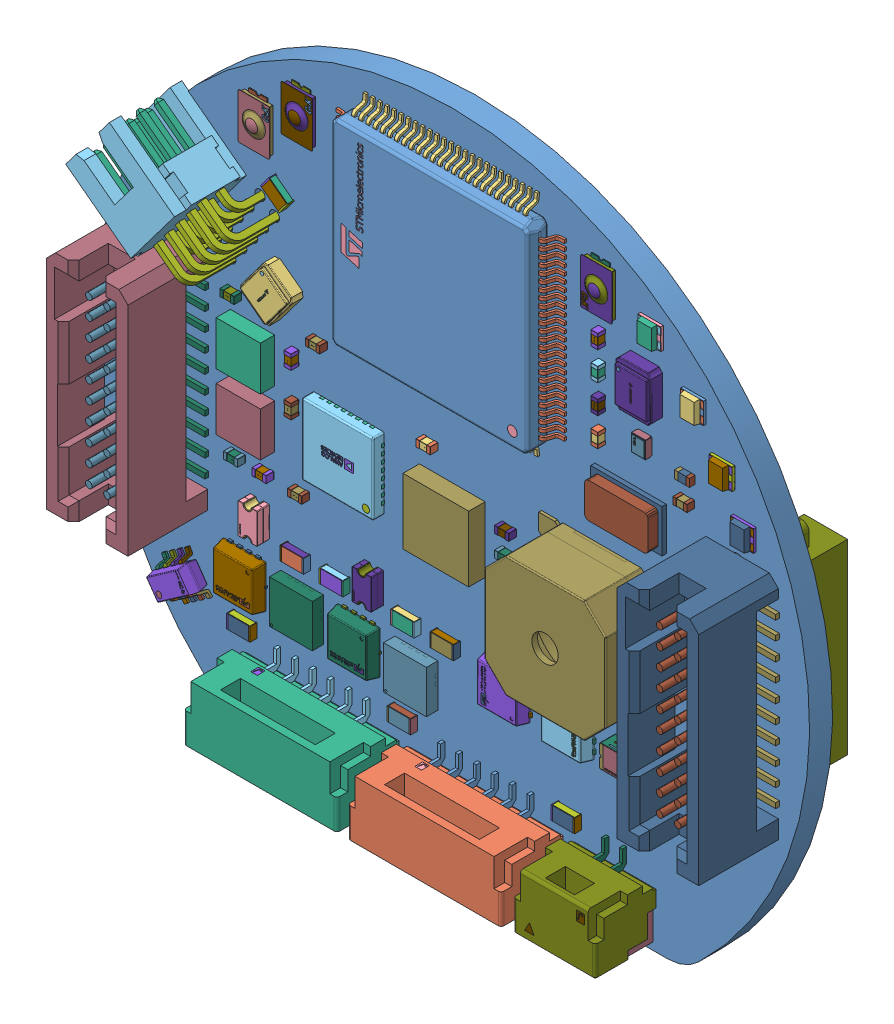
SolidWorks assembly HYDRA_V4_RECOVERY, configuration Default. Lengths in mm. (continued)
Components (placement in the parent): (continued)
- Open CASCADE STEP translator 7.5 3079-1: Open CASCADE STEP translator 7.5 3079 [Default] at origin size (0.1 0.95 0.5)
- Open CASCADE STEP translator 7.5 3080-1: Open CASCADE STEP translator 7.5 3080 [Default] at origin size (0.1 0.95 0.5)
- Open CASCADE STEP translator 7.5 3081-1: Open CASCADE STEP translator 7.5 3081 [Default] at origin size (1.45 0.95 0.05)
- Open CASCADE STEP translator 7.5 3082-1: Open CASCADE STEP translator 7.5 3082 [Default] at origin size (1.55 0.95 0.4)
- Open CASCADE STEP translator 7.5 3083-1: Open CASCADE STEP translator 7.5 3083 [Default] at origin size (0.1 0.95 0.5)
- Open CASCADE STEP translator 7.5 3084-1: Open CASCADE STEP translator 7.5 3084 [Default] at origin size (0.1 0.95 0.5)
- Open CASCADE STEP translator 7.5 3085-1: Open CASCADE STEP translator 7.5 3085 [Default] at origin size (1.45 0.95 0.05)
- Open CASCADE STEP translator 7.5 3086-1: Open CASCADE STEP translator 7.5 3086 [Default] at origin size (0.95 1.55 0.4)
- Open CASCADE STEP translator 7.5 3087-1: Open CASCADE STEP translator 7.5 3087 [Default] at origin size (0.95 0.1 0.5)
- Open CASCADE STEP translator 7.5 3088-1: Open CASCADE STEP translator 7.5 3088 [Default] at origin size (0.95 0.1 0.5)
- Open CASCADE STEP translator 7.5 3089-1: Open CASCADE STEP translator 7.5 3089 [Default] at origin size (0.95 1.45 0.05)
- Open CASCADE STEP translator 7.5 3090-1: Open CASCADE STEP translator 7.5 3090 [Default] at origin size (1.55 0.95 0.4)
- Open CASCADE STEP translator 7.5 3091-1: Open CASCADE STEP translator 7.5 3091 [Default] at origin size (0.1 0.95 0.5)
- Open CASCADE STEP translator 7.5 3092-1: Open CASCADE STEP translator 7.5 3092 [Default] at origin size (0.1 0.95 0.5)
- Open CASCADE STEP translator 7.5 3093-1: Open CASCADE STEP translator 7.5 3093 [Default] at origin size (1.45 0.95 0.05)
- Open CASCADE STEP translator 7.5 3094-1: Open CASCADE STEP translator 7.5 3094 [Default] at origin size (1.55 0.95 0.4)
- Open CASCADE STEP translator 7.5 3095-1: Open CASCADE STEP translator 7.5 3095 [Default] at origin size (0.1 0.95 0.5)
- Open CASCADE STEP translator 7.5 3096-1: Open CASCADE STEP translator 7.5 3096 [Default] at origin size (0.1 0.95 0.5)
- Open CASCADE STEP translator 7.5 3097-1: Open CASCADE STEP translator 7.5 3097 [Default] at origin size (1.45 0.95 0.05)
- Open CASCADE STEP translator 7.5 3098-1: Open CASCADE STEP translator 7.5 3098 [Default] at origin size (0.95 1.55 0.4)
- Open CASCADE STEP translator 7.5 3099-1: Open CASCADE STEP translator 7.5 3099 [Default] at origin size (0.95 0.1 0.5)
- Open CASCADE STEP translator 7.5 3100-1: Open CASCADE STEP translator 7.5 3100 [Default] at origin size (0.95 0.1 0.5)
- Open CASCADE STEP translator 7.5 3101-1: Open CASCADE STEP translator 7.5 3101 [Default] at origin size (0.95 1.45 0.05)
- Open CASCADE STEP translator 7.5 3102-1: Open CASCADE STEP translator 7.5 3102 [Default] at origin size (1.55 0.95 0.4)
- Open CASCADE STEP translator 7.5 3103-1: Open CASCADE STEP translator 7.5 3103 [Default] at origin size (0.1 0.95 0.5)
- Open CASCADE STEP translator 7.5 3104-1: Open CASCADE STEP translator 7.5 3104 [Default] at origin size (0.1 0.95 0.5)
- Open CASCADE STEP translator 7.5 3105-1: Open CASCADE STEP translator 7.5 3105 [Default] at origin size (1.45 0.95 0.05)
- Open CASCADE STEP translator 7.5 3106-1: Open CASCADE STEP translator 7.5 3106 [Default] at origin size (1.55 0.95 0.4)
- Open CASCADE STEP translator 7.5 3107-1: Open CASCADE STEP translator 7.5 3107 [Default] at origin size (0.1 0.95 0.5)
- Open CASCADE STEP translator 7.5 3108-1: Open CASCADE STEP translator 7.5 3108 [Default] at origin size (0.1 0.95 0.5)
- Open CASCADE STEP translator 7.5 3109-1: Open CASCADE STEP translator 7.5 3109 [Default] at origin size (1.45 0.95 0.05)
- Open CASCADE STEP translator 7.5 3110-1: Open CASCADE STEP translator 7.5 3110 [Default] at origin size (1.55 0.95 0.4)
- Open CASCADE STEP translator 7.5 3111-1: Open CASCADE STEP translator 7.5 3111 [Default] at origin size (0.1 0.95 0.5)
- Open CASCADE STEP translator 7.5 3112-1: Open CASCADE STEP translator 7.5 3112 [Default] at origin size (0.1 0.95 0.5)
- Open CASCADE STEP translator 7.5 3113-1: Open CASCADE STEP translator 7.5 3113 [Default] at origin size (1.45 0.95 0.05)
- Open CASCADE STEP translator 7.5 3114-1: Open CASCADE STEP translator 7.5 3114 [Default] at origin size (1.55 0.95 0.4)
- Open CASCADE STEP translator 7.5 3115-1: Open CASCADE STEP translator 7.5 3115 [Default] at origin size (0.1 0.95 0.5)
- Open CASCADE STEP translator 7.5 3116-1: Open CASCADE STEP translator 7.5 3116 [Default] at origin size (0.1 0.95 0.5)
- Open CASCADE STEP translator 7.5 3117-1: Open CASCADE STEP translator 7.5 3117 [Default] at origin size (1.45 0.95 0.05)
- Open CASCADE STEP translator 7.5 3118-1: Open CASCADE STEP translator 7.5 3118 [Default] at origin size (0.95 1.55 0.4)
- Open CASCADE STEP translator 7.5 3119-1: Open CASCADE STEP translator 7.5 3119 [Default] at origin size (0.95 0.1 0.5)
- Open CASCADE STEP translator 7.5 3120-1: Open CASCADE STEP translator 7.5 3120 [Default] at origin size (0.95 0.1 0.5)
- Open CASCADE STEP translator 7.5 3121-1: Open CASCADE STEP translator 7.5 3121 [Default] at origin size (0.95 1.45 0.05)
- Open CASCADE STEP translator 7.5 3122-1: Open CASCADE STEP translator 7.5 3122 [Default] at origin size (1.55 0.95 0.4)
- Open CASCADE STEP translator 7.5 3123-1: Open CASCADE STEP translator 7.5 3123 [Default] at origin size (0.1 0.95 0.5)
- Open CASCADE STEP translator 7.5 3124-1: Open CASCADE STEP translator 7.5 3124 [Default] at origin size (0.1 0.95 0.5)
- Open CASCADE STEP translator 7.5 3125-1: Open CASCADE STEP translator 7.5 3125 [Default] at origin size (1.45 0.95 0.05)
- Open CASCADE STEP translator 7.5 3126-1: Open CASCADE STEP translator 7.5 3126 [Default] at origin size (1.55 0.95 0.4)
- Open CASCADE STEP translator 7.5 3127-1: Open CASCADE STEP translator 7.5 3127 [Default] at origin size (0.1 0.95 0.5)
- Open CASCADE STEP translator 7.5 3128-1: Open CASCADE STEP translator 7.5 3128 [Default] at origin size (0.1 0.95 0.5)
- Open CASCADE STEP translator 7.5 3129-1: Open CASCADE STEP translator 7.5 3129 [Default] at origin size (1.45 0.95 0.05)
- Open CASCADE STEP translator 7.5 3130-1: Open CASCADE STEP translator 7.5 3130 [Default] at origin size (0.95 1.55 0.4)
- Open CASCADE STEP translator 7.5 3131-1: Open CASCADE STEP translator 7.5 3131 [Default] at origin size (0.95 0.1 0.5)
- Open CASCADE STEP translator 7.5 3132-1: Open CASCADE STEP translator 7.5 3132 [Default] at origin size (0.95 0.1 0.5)
- Open CASCADE STEP translator 7.5 3133-1: Open CASCADE STEP translator 7.5 3133 [Default] at origin size (0.95 1.45 0.05)
- Open CASCADE STEP translator 7.5 3134-1: Open CASCADE STEP translator 7.5 3134 [Default] at origin size (1.36 2.21 1.09)
- Open CASCADE STEP translator 7.5 3135-1: Open CASCADE STEP translator 7.5 3135 [Default] at origin size (0.43 0.4 0.59)
- Open CASCADE STEP translator 7.5 3136-1: Open CASCADE STEP translator 7.5 3136 [Default] at origin size (0.43 0.4 0.59)
- Open CASCADE STEP translator 7.5 3137-1: Open CASCADE STEP translator 7.5 3137 [Default] at origin size (0.43 0.4 0.59)
- Open CASCADE STEP translator 7.5 3138-1: Open CASCADE STEP translator 7.5 3138 [Default] at origin size (3 3 0.86)
- Open CASCADE STEP translator 7.5 3139-1: Open CASCADE STEP translator 7.5 3139 [Default] at origin size (3.2 3.1 0.15)
- Open CASCADE STEP translator 7.5 3140-1: Open CASCADE STEP translator 7.5 3140 [Default] at origin size (0.53 2.36 0.02)
- Open CASCADE STEP translator 7.5 3141-1: Open CASCADE STEP translator 7.5 3141 [Default] at origin size (3 3 0.86)
- Open CASCADE STEP translator 7.5 3142-1: Open CASCADE STEP translator 7.5 3142 [Default] at origin size (3.2 3.1 0.15)
- Open CASCADE STEP translator 7.5 3143-1: Open CASCADE STEP translator 7.5 3143 [Default] at origin size (0.53 2.36 0.02)
- Open CASCADE STEP translator 7.5 3144-1: Open CASCADE STEP translator 7.5 3144 [Default] at origin size (2.21 1.36 1.09)
- Open CASCADE STEP translator 7.5 3145-1: Open CASCADE STEP translator 7.5 3145 [Default] at origin size (0.4 0.43 0.59)
- Open CASCADE STEP translator 7.5 3146-1: Open CASCADE STEP translator 7.5 3146 [Default] at origin size (0.4 0.43 0.59)
- Open CASCADE STEP translator 7.5 3147-1: Open CASCADE STEP translator 7.5 3147 [Default] at origin size (0.4 0.43 0.59)
- Open CASCADE STEP translator 7.5 3148-1: Open CASCADE STEP translator 7.5 3148 [Default] at origin size (3 3 0.86)
- Open CASCADE STEP translator 7.5 3149-1: Open CASCADE STEP translator 7.5 3149 [Default] at origin size (3.1 3.2 0.15)
- Open CASCADE STEP translator 7.5 3150-1: Open CASCADE STEP translator 7.5 3150 [Default] at origin size (2.36 0.53 0.02)
- Open CASCADE STEP translator 7.5 3151-1: Open CASCADE STEP translator 7.5 3151 [Default] at origin size (1.25 2 0.96)
- Open CASCADE STEP translator 7.5 3152-1: Open CASCADE STEP translator 7.5 3152 [Default] at origin size (0.8 0.2 0.75)
- Open CASCADE STEP translator 7.5 3153-1: Open CASCADE STEP translator 7.5 3153 [Default] at origin size (0.8 0.2 0.75)
- Open CASCADE STEP translator 7.5 3154-1: Open CASCADE STEP translator 7.5 3154 [Default] at origin size (0.8 0.2 0.75)
- Open CASCADE STEP translator 7.5 3155-1: Open CASCADE STEP translator 7.5 3155 [Default] at origin size (0.25 0.25 0.01)
- Open CASCADE STEP translator 7.5 3156-1: Open CASCADE STEP translator 7.5 3156 [Default] at origin size (0.8 0.2 0.75)
- Open CASCADE STEP translator 7.5 3157-1: Open CASCADE STEP translator 7.5 3157 [Default] at origin size (0.8 0.2 0.75)
- Open CASCADE STEP translator 7.5 3158-1: Open CASCADE STEP translator 7.5 3158 [Default] at origin size (0.8 0.2 0.75)
- Open CASCADE STEP translator 7.5 3159-1: Open CASCADE STEP translator 7.5 3159 [Default] at origin size (0.96 0.16 0.01)
- Open CASCADE STEP translator 7.5 3160-1: Open CASCADE STEP translator 7.5 3160 [Default] at origin size (3 3 0.86)
- Open CASCADE STEP translator 7.5 3161-1: Open CASCADE STEP translator 7.5 3161 [Default] at origin size (3.1 3.2 0.15)
- Open CASCADE STEP translator 7.5 3162-1: Open CASCADE STEP translator 7.5 3162 [Default] at origin size (2.36 0.53 0.02)
- Open CASCADE STEP translator 7.5 3163-1: Open CASCADE STEP translator 7.5 3163 [Default] at origin size (8.53 8.53 4)
- Open CASCADE STEP translator 7.5 3164-1: Open CASCADE STEP translator 7.5 3164 [Default] at origin size (0.2 2.2 2.05)
- Open CASCADE STEP translator 7.5 3165-1: Open CASCADE STEP translator 7.5 3165 [Default] at origin size (0.2 2.2 2.05)
- Open CASCADE STEP translator 7.5 3166-1: Open CASCADE STEP translator 7.5 3166 [Default] at origin size (1.45 1.3 1.05)
- Open CASCADE STEP translator 7.5 3167-1: Open CASCADE STEP translator 7.5 3167 [Default] at origin size (5.75 4.05 4.25)
- Open CASCADE STEP translator 7.5 3168-1: Open CASCADE STEP translator 7.5 3168 [Default] at origin size (1.45 2.03 0.46)
- Open CASCADE STEP translator 7.5 3169-1: Open CASCADE STEP translator 7.5 3169 [Default] at origin size (4.2 3.06 0.01)
- Open CASCADE STEP translator 7.5 3170-1: Open CASCADE STEP translator 7.5 3170 [Default] at origin size (6.45 4.3 2.13)
- Open CASCADE STEP translator 7.5 3171-1: Open CASCADE STEP translator 7.5 3171 [Default] at origin size (10.75 4.05 4.35)
- Open CASCADE STEP translator 7.5 3172-1: Open CASCADE STEP translator 7.5 3172 [Default] at origin size (10.15 2.2 3)
- Open CASCADE STEP translator 7.5 3173-1: Open CASCADE STEP translator 7.5 3173 [Default] at origin size (0.46 0.01 0.54)
- Open CASCADE STEP translator 7.5 3174-1: Open CASCADE STEP translator 7.5 3174 [Default] at origin size (6.45 4.3 2.13)
- Open CASCADE STEP translator 7.5 3175-1: Open CASCADE STEP translator 7.5 3175 [Default] at origin size (10.75 4.05 4.35)
- Open CASCADE STEP translator 7.5 3176-1: Open CASCADE STEP translator 7.5 3176 [Default] at origin size (10.15 2.2 3)
- Open CASCADE STEP translator 7.5 3177-1: Open CASCADE STEP translator 7.5 3177 [Default] at origin size (0.46 0.01 0.54)
- Open CASCADE STEP translator 7.5 3178-1: Open CASCADE STEP translator 7.5 3178 [Default] at origin size (1 0.5 0.55)
- Open CASCADE STEP translator 7.5 3179-1: Open CASCADE STEP translator 7.5 3179 [Default] at origin size (0.5 0.49 0.54)
- Open CASCADE STEP translator 7.5 3180-1: Open CASCADE STEP translator 7.5 3180 [Default] at origin size (0.26 0.06 0.01)
- Open CASCADE STEP translator 7.5 3181-1: Open CASCADE STEP translator 7.5 3181 [Default] at origin size (3.2 1.6 1.1)
- Open CASCADE STEP translator 7.5 3182-1: Open CASCADE STEP translator 7.5 3182 [Default] at origin size (2.7 1.6 0.03)
- Open CASCADE STEP translator 7.5 3183-1: Open CASCADE STEP translator 7.5 3183 [Default] at origin size (2.7 1.6 0.03)
- Open CASCADE STEP translator 7.5 3184-1: Open CASCADE STEP translator 7.5 3184 [Default] at origin size (3.2 0.6 1.04)
- Open CASCADE STEP translator 7.5 3185-1: Open CASCADE STEP translator 7.5 3185 [Default] at origin size (3.2 0.6 1.04)
- Open CASCADE STEP translator 7.5 3186-1: Open CASCADE STEP translator 7.5 3186 [Default] at origin size (2.2 1.6 0.1)
- Open CASCADE STEP translator 7.5 3187-1: Open CASCADE STEP translator 7.5 3187 [Default] at origin size (2.2 1.6 0.1)
- Open CASCADE STEP translator 7.5 3188-1: Open CASCADE STEP translator 7.5 3188 [Default] at origin size (2.2 1.6 0.1)
- Open CASCADE STEP translator 7.5 3189-1: Open CASCADE STEP translator 7.5 3189 [Default] at origin size (1.21 0.16 0.02)
- Open CASCADE STEP translator 7.5 3190-1: Open CASCADE STEP translator 7.5 3190 [Default] at origin size (1.6 1.76 0.76)
- Open CASCADE STEP translator 7.5 3191-1: Open CASCADE STEP translator 7.5 3191 [Default] at origin size (1.59 1.75 0.75)
- Open CASCADE STEP translator 7.5 3192-1: Open CASCADE STEP translator 7.5 3192 [Default] at origin size (0.58 0.74 0.02)
- Open CASCADE STEP translator 7.5 3193-1: Open CASCADE STEP translator 7.5 3193 [Default] at origin size (0.85 1.66 0.99)
- Open CASCADE STEP translator 7.5 3194-1: Open CASCADE STEP translator 7.5 3194 [Default] at origin size (0.85 0.5 0.01)
- Open CASCADE STEP translator 7.5 3195-1: Open CASCADE STEP translator 7.5 3195 [Default] at origin size (0.83 0.11 0)
- Open CASCADE STEP translator 7.5 3196-1: Open CASCADE STEP translator 7.5 3196 [Default] at origin size (0.85 0.5 0.01)
- Open CASCADE STEP translator 7.5 3197-1: Open CASCADE STEP translator 7.5 3197 [Default] at origin size (0.85 1.66 0.99)
- Open CASCADE STEP translator 7.5 3198-1: Open CASCADE STEP translator 7.5 3198 [Default] at origin size (0.85 0.5 0.01)
- Open CASCADE STEP translator 7.5 3199-1: Open CASCADE STEP translator 7.5 3199 [Default] at origin size (0.83 0.11 0)
- Open CASCADE STEP translator 7.5 3200-1: Open CASCADE STEP translator 7.5 3200 [Default] at origin size (0.85 0.5 0.01)
- Open CASCADE STEP translator 7.5 3201-1: Open CASCADE STEP translator 7.5 3201 [Default] at origin size (1.35 0.95 0.01)
- Open CASCADE STEP translator 7.5 3202-1: Open CASCADE STEP translator 7.5 3202 [Default] at origin size (1.35 2.15 0.01)
- Open CASCADE STEP translator 7.5 3203-1: Open CASCADE STEP translator 7.5 3203 [Default] at origin size (0.65 2.16 0.85)
- Open CASCADE STEP translator 7.5 3204-1: Open CASCADE STEP translator 7.5 3204 [Default] at origin size (1.35 2.15 0.85)
- Open CASCADE STEP translator 7.5 3205-1: Open CASCADE STEP translator 7.5 3205 [Default] at origin size (0.09 0.66 0.02)
- Open CASCADE STEP translator 7.5 3206-1: Open CASCADE STEP translator 7.5 3206 [Default] at origin size (1.35 0.95 0.01)
- Open CASCADE STEP translator 7.5 3207-1: Open CASCADE STEP translator 7.5 3207 [Default] at origin size (1.35 2.15 0.01)
- Open CASCADE STEP translator 7.5 3208-1: Open CASCADE STEP translator 7.5 3208 [Default] at origin size (0.65 2.16 0.85)
- Open CASCADE STEP translator 7.5 3209-1: Open CASCADE STEP translator 7.5 3209 [Default] at origin size (1.35 2.15 0.85)
- Open CASCADE STEP translator 7.5 3210-1: Open CASCADE STEP translator 7.5 3210 [Default] at origin size (0.09 0.66 0.02)
- Open CASCADE STEP translator 7.5 3211-1: Open CASCADE STEP translator 7.5 3211 [Default] at origin size (1.2 0.8 0.7)
- Open CASCADE STEP translator 7.5 3212-1: Open CASCADE STEP translator 7.5 3212 [Default] at origin size (4.32 2.6 2.15)
- Open CASCADE STEP translator 7.5 3213-1: Open CASCADE STEP translator 7.5 3213 [Default] at origin size (1 0.5 0.55)
- Open CASCADE STEP translator 7.5 3214-1: Open CASCADE STEP translator 7.5 3214 [Default] at origin size (0.5 0.47 0.52)
- Open CASCADE STEP translator 7.5 3215-1: Open CASCADE STEP translator 7.5 3215 [Default] at origin size (0.3 0.03 0)
- Open CASCADE STEP translator 7.5 3216-1: Open CASCADE STEP translator 7.5 3216 [Default] at origin size (0.5 1 0.55)
- Open CASCADE STEP translator 7.5 3217-1: Open CASCADE STEP translator 7.5 3217 [Default] at origin size (0.47 0.5 0.52)
- Open CASCADE STEP translator 7.5 3218-1: Open CASCADE STEP translator 7.5 3218 [Default] at origin size (0.03 0.3 0)
- Open CASCADE STEP translator 7.5 3219-1: Open CASCADE STEP translator 7.5 3219 [Default] at origin size (1.1 1 0.56)
- Open CASCADE STEP translator 7.5 3220-1: Open CASCADE STEP translator 7.5 3220 [Default] at origin size (0.68 0.68 0.52)
- Open CASCADE STEP translator 7.5 3221-1: Open CASCADE STEP translator 7.5 3221 [Default] at origin size (0.26 0.2 0)
- Open CASCADE STEP translator 7.5 3222-1: Open CASCADE STEP translator 7.5 3222 [Default] at origin size (1.1 1 0.56)
- Open CASCADE STEP translator 7.5 3223-1: Open CASCADE STEP translator 7.5 3223 [Default] at origin size (0.68 0.68 0.52)
- Open CASCADE STEP translator 7.5 3224-1: Open CASCADE STEP translator 7.5 3224 [Default] at origin size (0.26 0.2 0)
- Open CASCADE STEP translator 7.5 3225-1: Open CASCADE STEP translator 7.5 3225 [Default] at origin size (1 1.1 0.56)
- Open CASCADE STEP translator 7.5 3226-1: Open CASCADE STEP translator 7.5 3226 [Default] at origin size (0.68 0.68 0.52)
- Open CASCADE STEP translator 7.5 3227-1: Open CASCADE STEP translator 7.5 3227 [Default] at origin size (0.2 0.25 0)
- Open CASCADE STEP translator 7.5 3228-1: Open CASCADE STEP translator 7.5 3228 [Default] at origin size (0.5 1 0.55)
- Open CASCADE STEP translator 7.5 3229-1: Open CASCADE STEP translator 7.5 3229 [Default] at origin size (0.47 0.5 0.52)
- Open CASCADE STEP translator 7.5 3230-1: Open CASCADE STEP translator 7.5 3230 [Default] at origin size (0.03 0.3 0)
- Open CASCADE STEP translator 7.5 3231-1: Open CASCADE STEP translator 7.5 3231 [Default] at origin size (0.5 1 0.55)
- Open CASCADE STEP translator 7.5 3232-1: Open CASCADE STEP translator 7.5 3232 [Default] at origin size (0.47 0.5 0.52)
- Open CASCADE STEP translator 7.5 3233-1: Open CASCADE STEP translator 7.5 3233 [Default] at origin size (0.03 0.3 0)
- Open CASCADE STEP translator 7.5 3234-1: Open CASCADE STEP translator 7.5 3234 [Default] at origin size (0.5 1 0.55)
- Open CASCADE STEP translator 7.5 3235-1: Open CASCADE STEP translator 7.5 3235 [Default] at origin size (0.47 0.5 0.52)
- Open CASCADE STEP translator 7.5 3236-1: Open CASCADE STEP translator 7.5 3236 [Default] at origin size (0.03 0.3 0)
- Open CASCADE STEP translator 7.5 3237-1: Open CASCADE STEP translator 7.5 3237 [Default] at origin size (0.5 1 0.55)
- Open CASCADE STEP translator 7.5 3238-1: Open CASCADE STEP translator 7.5 3238 [Default] at origin size (0.47 0.5 0.52)
- Open CASCADE STEP translator 7.5 3239-1: Open CASCADE STEP translator 7.5 3239 [Default] at origin size (0.03 0.3 0)
- Open CASCADE STEP translator 7.5 3240-1: Open CASCADE STEP translator 7.5 3240 [Default] at origin size (0.5 1 0.55)
- Open CASCADE STEP translator 7.5 3241-1: Open CASCADE STEP translator 7.5 3241 [Default] at origin size (0.47 0.5 0.52)
- Open CASCADE STEP translator 7.5 3242-1: Open CASCADE STEP translator 7.5 3242 [Default] at origin size (0.03 0.3 0)
- Open CASCADE STEP translator 7.5 3243-1: Open CASCADE STEP translator 7.5 3243 [Default] at origin size (0.5 1 0.55)
- Open CASCADE STEP translator 7.5 3244-1: Open CASCADE STEP translator 7.5 3244 [Default] at origin size (0.47 0.5 0.52)
- Open CASCADE STEP translator 7.5 3245-1: Open CASCADE STEP translator 7.5 3245 [Default] at origin size (0.03 0.3 0)
- Open CASCADE STEP translator 7.5 3246-1: Open CASCADE STEP translator 7.5 3246 [Default] at origin size (0.5 1 0.55)
- Open CASCADE STEP translator 7.5 3247-1: Open CASCADE STEP translator 7.5 3247 [Default] at origin size (0.47 0.5 0.52)
- Open CASCADE STEP translator 7.5 3248-1: Open CASCADE STEP translator 7.5 3248 [Default] at origin size (0.03 0.3 0)
- Open CASCADE STEP translator 7.5 3249-1: Open CASCADE STEP translator 7.5 3249 [Default] at origin size (0.5 1 0.55)
- Open CASCADE STEP translator 7.5 3250-1: Open CASCADE STEP translator 7.5 3250 [Default] at origin size (0.47 0.5 0.52)
- Open CASCADE STEP translator 7.5 3251-1: Open CASCADE STEP translator 7.5 3251 [Default] at origin size (0.03 0.3 0)
- Open CASCADE STEP translator 7.5 3252-1: Open CASCADE STEP translator 7.5 3252 [Default] at origin size (0.5 1 0.55)
- Open CASCADE STEP translator 7.5 3253-1: Open CASCADE STEP translator 7.5 3253 [Default] at origin size (0.47 0.5 0.52)
- Open CASCADE STEP translator 7.5 3254-1: Open CASCADE STEP translator 7.5 3254 [Default] at origin size (0.03 0.3 0)
- Open CASCADE STEP translator 7.5 3255-1: Open CASCADE STEP translator 7.5 3255 [Default] at origin size (0.5 1 0.55)
- Open CASCADE STEP translator 7.5 3256-1: Open CASCADE STEP translator 7.5 3256 [Default] at origin size (0.47 0.5 0.52)
- Open CASCADE STEP translator 7.5 3257-1: Open CASCADE STEP translator 7.5 3257 [Default] at origin size (0.03 0.3 0)
- Open CASCADE STEP translator 7.5 3258-1: Open CASCADE STEP translator 7.5 3258 [Default] at origin size (0.5 1 0.55)
- Open CASCADE STEP translator 7.5 3259-1: Open CASCADE STEP translator 7.5 3259 [Default] at origin size (0.47 0.5 0.52)
- Open CASCADE STEP translator 7.5 3260-1: Open CASCADE STEP translator 7.5 3260 [Default] at origin size (0.03 0.3 0)
- Open CASCADE STEP translator 7.5 3261-1: Open CASCADE STEP translator 7.5 3261 [Default] at origin size (1 0.5 0.55)
- Open CASCADE STEP translator 7.5 3262-1: Open CASCADE STEP translator 7.5 3262 [Default] at origin size (0.5 0.47 0.52)
- Open CASCADE STEP translator 7.5 3263-1: Open CASCADE STEP translator 7.5 3263 [Default] at origin size (0.3 0.03 0)
- Open CASCADE STEP translator 7.5 3264-1: Open CASCADE STEP translator 7.5 3264 [Default] at origin size (0.5 1 0.55)
- Open CASCADE STEP translator 7.5 3265-1: Open CASCADE STEP translator 7.5 3265 [Default] at origin size (0.47 0.5 0.52)
- Open CASCADE STEP translator 7.5 3266-1: Open CASCADE STEP translator 7.5 3266 [Default] at origin size (0.03 0.3 0)
- Open CASCADE STEP translator 7.5 3267-1: Open CASCADE STEP translator 7.5 3267 [Default] at origin size (0.5 1 0.55)
- Open CASCADE STEP translator 7.5 3268-1: Open CASCADE STEP translator 7.5 3268 [Default] at origin size (0.47 0.5 0.52)
- Open CASCADE STEP translator 7.5 3269-1: Open CASCADE STEP translator 7.5 3269 [Default] at origin size (0.03 0.3 0)
- Open CASCADE STEP translator 7.5 3270-1: Open CASCADE STEP translator 7.5 3270 [Default] at origin size (0.5 1 0.55)
- Open CASCADE STEP translator 7.5 3271-1: Open CASCADE STEP translator 7.5 3271 [Default] at origin size (0.47 0.5 0.52)
- Open CASCADE STEP translator 7.5 3272-1: Open CASCADE STEP translator 7.5 3272 [Default] at origin size (0.03 0.3 0)
- Open CASCADE STEP translator 7.5 3273-1: Open CASCADE STEP translator 7.5 3273 [Default] at origin size (0.5 1 0.55)
- Open CASCADE STEP translator 7.5 3274-1: Open CASCADE STEP translator 7.5 3274 [Default] at origin size (0.47 0.5 0.52)
- Open CASCADE STEP translator 7.5 3275-1: Open CASCADE STEP translator 7.5 3275 [Default] at origin size (0.03 0.3 0)
- Open CASCADE STEP translator 7.5 3276-1: Open CASCADE STEP translator 7.5 3276 [Default] at origin size (0.5 1 0.55)
- Open CASCADE STEP translator 7.5 3277-1: Open CASCADE STEP translator 7.5 3277 [Default] at origin size (0.47 0.5 0.52)
- Open CASCADE STEP translator 7.5 3278-1: Open CASCADE STEP translator 7.5 3278 [Default] at origin size (0.03 0.3 0)
- Open CASCADE STEP translator 7.5 3279-1: Open CASCADE STEP translator 7.5 3279 [Default] at origin size (0.5 1 0.55)
- Open CASCADE STEP translator 7.5 3280-1: Open CASCADE STEP translator 7.5 3280 [Default] at origin size (0.47 0.5 0.52)
- Open CASCADE STEP translator 7.5 3281-1: Open CASCADE STEP translator 7.5 3281 [Default] at origin size (0.03 0.3 0)
- Open CASCADE STEP translator 7.5 3282-1: Open CASCADE STEP translator 7.5 3282 [Default] at origin size (0.5 1 0.55)
- Open CASCADE STEP translator 7.5 3283-1: Open CASCADE STEP translator 7.5 3283 [Default] at origin size (0.47 0.5 0.52)
- Open CASCADE STEP translator 7.5 3284-1: Open CASCADE STEP translator 7.5 3284 [Default] at origin size (0.03 0.3 0)
- Open CASCADE STEP translator 7.5 3285-1: Open CASCADE STEP translator 7.5 3285 [Default] at origin size (0.5 1 0.55)
- Open CASCADE STEP translator 7.5 3286-1: Open CASCADE STEP translator 7.5 3286 [Default] at origin size (0.47 0.5 0.52)
- Open CASCADE STEP translator 7.5 3287-1: Open CASCADE STEP translator 7.5 3287 [Default] at origin size (0.03 0.3 0)
- Open CASCADE STEP translator 7.5 3288-1: Open CASCADE STEP translator 7.5 3288 [Default] at origin size (0.5 1 0.55)
- Open CASCADE STEP translator 7.5 3289-1: Open CASCADE STEP translator 7.5 3289 [Default] at origin size (0.47 0.5 0.52)
- Open CASCADE STEP translator 7.5 3290-1: Open CASCADE STEP translator 7.5 3290 [Default] at origin size (0.03 0.3 0)
- Open CASCADE STEP translator 7.5 3291-1: Open CASCADE STEP translator 7.5 3291 [Default] at origin size (1 0.5 0.55)
- Open CASCADE STEP translator 7.5 3292-1: Open CASCADE STEP translator 7.5 3292 [Default] at origin size (0.5 0.47 0.52)
- Open CASCADE STEP translator 7.5 3293-1: Open CASCADE STEP translator 7.5 3293 [Default] at origin size (0.3 0.03 0)
- Open CASCADE STEP translator 7.5 3294-1: Open CASCADE STEP translator 7.5 3294 [Default] at origin size (1 0.5 0.55)
- Open CASCADE STEP translator 7.5 3295-1: Open CASCADE STEP translator 7.5 3295 [Default] at origin size (0.5 0.47 0.52)
- Open CASCADE STEP translator 7.5 3296-1: Open CASCADE STEP translator 7.5 3296 [Default] at origin size (0.3 0.03 0)
- Open CASCADE STEP translator 7.5 3297-1: Open CASCADE STEP translator 7.5 3297 [Default] at origin size (0.5 1 0.55)
- Open CASCADE STEP translator 7.5 3298-1: Open CASCADE STEP translator 7.5 3298 [Default] at origin size (0.47 0.5 0.52)
- Open CASCADE STEP translator 7.5 3299-1: Open CASCADE STEP translator 7.5 3299 [Default] at origin size (0.03 0.3 0)
- Open CASCADE STEP translator 7.5 3300-1: Open CASCADE STEP translator 7.5 3300 [Default] at origin size (0.5 1 0.55)
- Open CASCADE STEP translator 7.5 3301-1: Open CASCADE STEP translator 7.5 3301 [Default] at origin size (0.47 0.5 0.52)
- Open CASCADE STEP translator 7.5 3302-1: Open CASCADE STEP translator 7.5 3302 [Default] at origin size (0.03 0.3 0)
- Open CASCADE STEP translator 7.5 3303-1: Open CASCADE STEP translator 7.5 3303 [Default] at origin size (1 0.5 0.55)
- Open CASCADE STEP translator 7.5 3304-1: Open CASCADE STEP translator 7.5 3304 [Default] at origin size (0.5 0.47 0.52)
- Open CASCADE STEP translator 7.5 3305-1: Open CASCADE STEP translator 7.5 3305 [Default] at origin size (0.3 0.03 0)
- Open CASCADE STEP translator 7.5 3306-1: Open CASCADE STEP translator 7.5 3306 [Default] at origin size (1 0.5 0.55)
- Open CASCADE STEP translator 7.5 3307-1: Open CASCADE STEP translator 7.5 3307 [Default] at origin size (0.5 0.47 0.52)
- Open CASCADE STEP translator 7.5 3308-1: Open CASCADE STEP translator 7.5 3308 [Default] at origin size (0.3 0.03 0)
- Open CASCADE STEP translator 7.5 3309-1: Open CASCADE STEP translator 7.5 3309 [Default] at origin size (0.5 1 0.55)
- Open CASCADE STEP translator 7.5 3310-1: Open CASCADE STEP translator 7.5 3310 [Default] at origin size (0.47 0.5 0.52)
- Open CASCADE STEP translator 7.5 3311-1: Open CASCADE STEP translator 7.5 3311 [Default] at origin size (0.03 0.3 0)
- Open CASCADE STEP translator 7.5 3312-1: Open CASCADE STEP translator 7.5 3312 [Default] at origin size (0.5 1 0.55)
- Open CASCADE STEP translator 7.5 3313-1: Open CASCADE STEP translator 7.5 3313 [Default] at origin size (0.47 0.5 0.52)
- Open CASCADE STEP translator 7.5 3314-1: Open CASCADE STEP translator 7.5 3314 [Default] at origin size (0.03 0.3 0)
- Open CASCADE STEP translator 7.5 3315-1: Open CASCADE STEP translator 7.5 3315 [Default] at origin size (1 0.5 0.55)
- Open CASCADE STEP translator 7.5 3316-1: Open CASCADE STEP translator 7.5 3316 [Default] at origin size (0.5 0.47 0.52)
- Open CASCADE STEP translator 7.5 3317-1: Open CASCADE STEP translator 7.5 3317 [Default] at origin size (0.3 0.03 0)
- Open CASCADE STEP translator 7.5 3318-1: Open CASCADE STEP translator 7.5 3318 [Default] at origin size (1 0.5 0.55)
- Open CASCADE STEP translator 7.5 3319-1: Open CASCADE STEP translator 7.5 3319 [Default] at origin size (0.5 0.47 0.52)
- Open CASCADE STEP translator 7.5 3320-1: Open CASCADE STEP translator 7.5 3320 [Default] at origin size (0.3 0.03 0)
- Open CASCADE STEP translator 7.5 3321-1: Open CASCADE STEP translator 7.5 3321 [Default] at origin size (0.5 1 0.55)
- Open CASCADE STEP translator 7.5 3322-1: Open CASCADE STEP translator 7.5 3322 [Default] at origin size (0.47 0.5 0.52)
- Open CASCADE STEP translator 7.5 3323-1: Open CASCADE STEP translator 7.5 3323 [Default] at origin size (0.03 0.3 0)
- Open CASCADE STEP translator 7.5 3324-1: Open CASCADE STEP translator 7.5 3324 [Default] at origin size (1 0.5 0.55)
- Open CASCADE STEP translator 7.5 3325-1: Open CASCADE STEP translator 7.5 3325 [Default] at origin size (0.5 0.47 0.52)
- Open CASCADE STEP translator 7.5 3326-1: Open CASCADE STEP translator 7.5 3326 [Default] at origin size (0.3 0.03 0)
- Open CASCADE STEP translator 7.5 3327-1: Open CASCADE STEP translator 7.5 3327 [Default] at origin size (1 0.5 0.55)
- Open CASCADE STEP translator 7.5 3328-1: Open CASCADE STEP translator 7.5 3328 [Default] at origin size (0.5 0.47 0.52)
- Open CASCADE STEP translator 7.5 3329-1: Open CASCADE STEP translator 7.5 3329 [Default] at origin size (0.3 0.03 0)
- Open CASCADE STEP translator 7.5 3330-1: Open CASCADE STEP translator 7.5 3330 [Default] at origin size (0.5 1 0.55)
- Open CASCADE STEP translator 7.5 3331-1: Open CASCADE STEP translator 7.5 3331 [Default] at origin size (0.47 0.5 0.52)
- Open CASCADE STEP translator 7.5 3332-1: Open CASCADE STEP translator 7.5 3332 [Default] at origin size (0.03 0.3 0)
- Open CASCADE STEP translator 7.5 3333-1: Open CASCADE STEP translator 7.5 3333 [Default] at origin size (1 0.5 0.55)
- Open CASCADE STEP translator 7.5 3334-1: Open CASCADE STEP translator 7.5 3334 [Default] at origin size (0.5 0.47 0.52)
- Open CASCADE STEP translator 7.5 3335-1: Open CASCADE STEP translator 7.5 3335 [Default] at origin size (0.3 0.03 0)
- Open CASCADE STEP translator 7.5 3336-1: Open CASCADE STEP translator 7.5 3336 [Default] at origin size (0.81 1.61 0.91)
- Open CASCADE STEP translator 7.5 3337-1: Open CASCADE STEP translator 7.5 3337 [Default] at origin size (0.8 0.85 0.9)
- Open CASCADE STEP translator 7.5 3338-1: Open CASCADE STEP translator 7.5 3338 [Default] at origin size (0.13 0.52 0.01)
- Open CASCADE STEP translator 7.5 3339-1: Open CASCADE STEP translator 7.5 3339 [Default] at origin size (1 0.5 0.55)
- Open CASCADE STEP translator 7.5 3340-1: Open CASCADE STEP translator 7.5 3340 [Default] at origin size (0.5 0.47 0.52)
- Open CASCADE STEP translator 7.5 3341-1: Open CASCADE STEP translator 7.5 3341 [Default] at origin size (0.3 0.03 0)
- Open CASCADE STEP translator 7.5 3342-1: Open CASCADE STEP translator 7.5 3342 [Default] at origin size (1 0.5 0.55)
- Open CASCADE STEP translator 7.5 3343-1: Open CASCADE STEP translator 7.5 3343 [Default] at origin size (0.5 0.47 0.52)
- Open CASCADE STEP translator 7.5 3344-1: Open CASCADE STEP translator 7.5 3344 [Default] at origin size (0.3 0.03 0)
- Open CASCADE STEP translator 7.5 3345-1: Open CASCADE STEP translator 7.5 3345 [Default] at origin size (1 0.5 0.55)
- Open CASCADE STEP translator 7.5 3346-1: Open CASCADE STEP translator 7.5 3346 [Default] at origin size (0.5 0.47 0.52)
- Open CASCADE STEP translator 7.5 3347-1: Open CASCADE STEP translator 7.5 3347 [Default] at origin size (0.3 0.03 0)
- Open CASCADE STEP translator 7.5 3348-1: Open CASCADE STEP translator 7.5 3348 [Default] at origin size (1 0.5 0.55)
- Open CASCADE STEP translator 7.5 3349-1: Open CASCADE STEP translator 7.5 3349 [Default] at origin size (0.5 0.47 0.52)
- Open CASCADE STEP translator 7.5 3350-1: Open CASCADE STEP translator 7.5 3350 [Default] at origin size (0.3 0.03 0)
- Open CASCADE STEP translator 7.5 3351-1: Open CASCADE STEP translator 7.5 3351 [Default] at origin size (1 0.5 0.55)
- Open CASCADE STEP translator 7.5 3352-1: Open CASCADE STEP translator 7.5 3352 [Default] at origin size (0.5 0.47 0.52)
- Open CASCADE STEP translator 7.5 3353-1: Open CASCADE STEP translator 7.5 3353 [Default] at origin size (0.3 0.03 0)
- Open CASCADE STEP translator 7.5 3354-1: Open CASCADE STEP translator 7.5 3354 [Default] at origin size (1 0.5 0.55)
- Open CASCADE STEP translator 7.5 3355-1: Open CASCADE STEP translator 7.5 3355 [Default] at origin size (0.5 0.47 0.52)
- Open CASCADE STEP translator 7.5 3356-1: Open CASCADE STEP translator 7.5 3356 [Default] at origin size (0.3 0.03 0)
- Open CASCADE STEP translator 7.5 3357-1: Open CASCADE STEP translator 7.5 3357 [Default] at origin size (1 0.5 0.55)
- Open CASCADE STEP translator 7.5 3358-1: Open CASCADE STEP translator 7.5 3358 [Default] at origin size (0.5 0.47 0.52)
- Open CASCADE STEP translator 7.5 3359-1: Open CASCADE STEP translator 7.5 3359 [Default] at origin size (0.3 0.03 0)
- Open CASCADE STEP translator 7.5 3360-1: Open CASCADE STEP translator 7.5 3360 [Default] at origin size (1 0.5 0.55)
- Open CASCADE STEP translator 7.5 3361-1: Open CASCADE STEP translator 7.5 3361 [Default] at origin size (0.5 0.47 0.52)
- Open CASCADE STEP translator 7.5 3362-1: Open CASCADE STEP translator 7.5 3362 [Default] at origin size (0.3 0.03 0)
- Open CASCADE STEP translator 7.5 3363-1: Open CASCADE STEP translator 7.5 3363 [Default] at origin size (1 0.5 0.55)
- Open CASCADE STEP translator 7.5 3364-1: Open CASCADE STEP translator 7.5 3364 [Default] at origin size (0.5 0.47 0.52)
- Open CASCADE STEP translator 7.5 3365-1: Open CASCADE STEP translator 7.5 3365 [Default] at origin size (0.3 0.03 0)
- Open CASCADE STEP translator 7.5 3366-1: Open CASCADE STEP translator 7.5 3366 [Default] at origin size (0.5 1 0.55)
- Open CASCADE STEP translator 7.5 3367-1: Open CASCADE STEP translator 7.5 3367 [Default] at origin size (0.47 0.5 0.52)
- Open CASCADE STEP translator 7.5 3368-1: Open CASCADE STEP translator 7.5 3368 [Default] at origin size (0.03 0.3 0)
- Open CASCADE STEP translator 7.5 3369-1: Open CASCADE STEP translator 7.5 3369 [Default] at origin size (0.5 1 0.55)
- Open CASCADE STEP translator 7.5 3370-1: Open CASCADE STEP translator 7.5 3370 [Default] at origin size (0.47 0.5 0.52)
- Open CASCADE STEP translator 7.5 3371-1: Open CASCADE STEP translator 7.5 3371 [Default] at origin size (0.03 0.3 0)
- Open CASCADE STEP translator 7.5 3372-1: Open CASCADE STEP translator 7.5 3372 [Default] at origin size (7.98 7.97 5.08)
- Open CASCADE STEP translator 7.5 3373-1: Open CASCADE STEP translator 7.5 3373 [Default] at origin size (6.65 6.86 1.68)
- Open CASCADE STEP translator 7.5 3374-1: Open CASCADE STEP translator 7.5 3374 [Default] at origin size (6.1 6.49 5.65)
- Open CASCADE STEP translator 7.5 3375-1: Open CASCADE STEP translator 7.5 3375 [Default] at origin size (1.6 1.5 0.2)
- Open CASCADE STEP translator 7.5 3376-1: Open CASCADE STEP translator 7.5 3376 [Default] at origin size (1.6 1.4 0.19)
- Open CASCADE STEP translator 7.5 3377-1: Open CASCADE STEP translator 7.5 3377 [Default] at origin size (1.1 1.5 0.36)
- Open CASCADE STEP translator 7.5 3378-1: Open CASCADE STEP translator 7.5 3378 [Default] at origin size (1.3 3.5 0.06)
- Open CASCADE STEP translator 7.5 3379-1: Open CASCADE STEP translator 7.5 3379 [Default] at origin size (2 3 0.57)
- Open CASCADE STEP translator 7.5 3380-1: Open CASCADE STEP translator 7.5 3380 [Default] at origin size (2.2 3.2 0.32)
- Open CASCADE STEP translator 7.5 3381-1: Open CASCADE STEP translator 7.5 3381 [Default] at origin size (0.46 0.93 0.01)
- Open CASCADE STEP translator 7.5 3382-1: Open CASCADE STEP translator 7.5 3382 [Default] at origin size (1.3 3.5 0.06)
- Open CASCADE STEP translator 7.5 3383-1: Open CASCADE STEP translator 7.5 3383 [Default] at origin size (2 3 0.57)
- Open CASCADE STEP translator 7.5 3384-1: Open CASCADE STEP translator 7.5 3384 [Default] at origin size (2.2 3.2 0.32)
- Open CASCADE STEP translator 7.5 3385-1: Open CASCADE STEP translator 7.5 3385 [Default] at origin size (0.46 0.93 0.01)
- Open CASCADE STEP translator 7.5 3386-1: Open CASCADE STEP translator 7.5 3386 [Default] at origin size (1.6 1.5 0.2)
- Open CASCADE STEP translator 7.5 3387-1: Open CASCADE STEP translator 7.5 3387 [Default] at origin size (1.6 1.4 0.19)
- Open CASCADE STEP translator 7.5 3388-1: Open CASCADE STEP translator 7.5 3388 [Default] at origin size (1.1 1.5 0.36)
- Open CASCADE STEP translator 7.5 3389-1: Open CASCADE STEP translator 7.5 3389 [Default] at origin size (1.6 1.5 0.2)
- Open CASCADE STEP translator 7.5 3390-1: Open CASCADE STEP translator 7.5 3390 [Default] at origin size (1.6 1.4 0.19)
- Open CASCADE STEP translator 7.5 3391-1: Open CASCADE STEP translator 7.5 3391 [Default] at origin size (1.1 1.5 0.36)
- Open CASCADE STEP translator 7.5 3392-1: Open CASCADE STEP translator 7.5 3392 [Default] at origin size (1.6 1.5 0.2)
- Open CASCADE STEP translator 7.5 3393-1: Open CASCADE STEP translator 7.5 3393 [Default] at origin size (1.6 1.4 0.19)
- Open CASCADE STEP translator 7.5 3394-1: Open CASCADE STEP translator 7.5 3394 [Default] at origin size (1.1 1.5 0.36)
- Open CASCADE STEP translator 7.5 3395-1: Open CASCADE STEP translator 7.5 3395 [Default] at origin size (5.72 15.88 6.73)
- Open CASCADE STEP translator 7.5 3396-1: Open CASCADE STEP translator 7.5 3396 [Default] at origin size (1.78 12.7 4.01)
- Open CASCADE STEP translator 7.5 3397-1: Open CASCADE STEP translator 7.5 3397 [Default] at origin size (5.84 12.7 0.83)
- Open CASCADE STEP translator 7.5 3398-1: Open CASCADE STEP translator 7.5 3398 [Default] at origin size (5.72 15.88 6.73)
- Open CASCADE STEP translator 7.5 3399-1: Open CASCADE STEP translator 7.5 3399 [Default] at origin size (1.78 12.7 4.01)
- Open CASCADE STEP translator 7.5 3400-1: Open CASCADE STEP translator 7.5 3400 [Default] at origin size (5.84 12.7 0.83)
- Open CASCADE STEP translator 7.5 3401-1: Open CASCADE STEP translator 7.5 3401 [Default] at origin size (3.68 15.88 5.84)
- Open CASCADE STEP translator 7.5 3402-1: Open CASCADE STEP translator 7.5 3402 [Default] at origin size (4.09 12.7 1.18)
- Open CASCADE STEP translator 7.5 3403-1: Open CASCADE STEP translator 7.5 3403 [Default] at origin size (3.68 15.88 5.84)
- Open CASCADE STEP translator 7.5 3404-1: Open CASCADE STEP translator 7.5 3404 [Default] at origin size (4.09 12.7 1.18)
